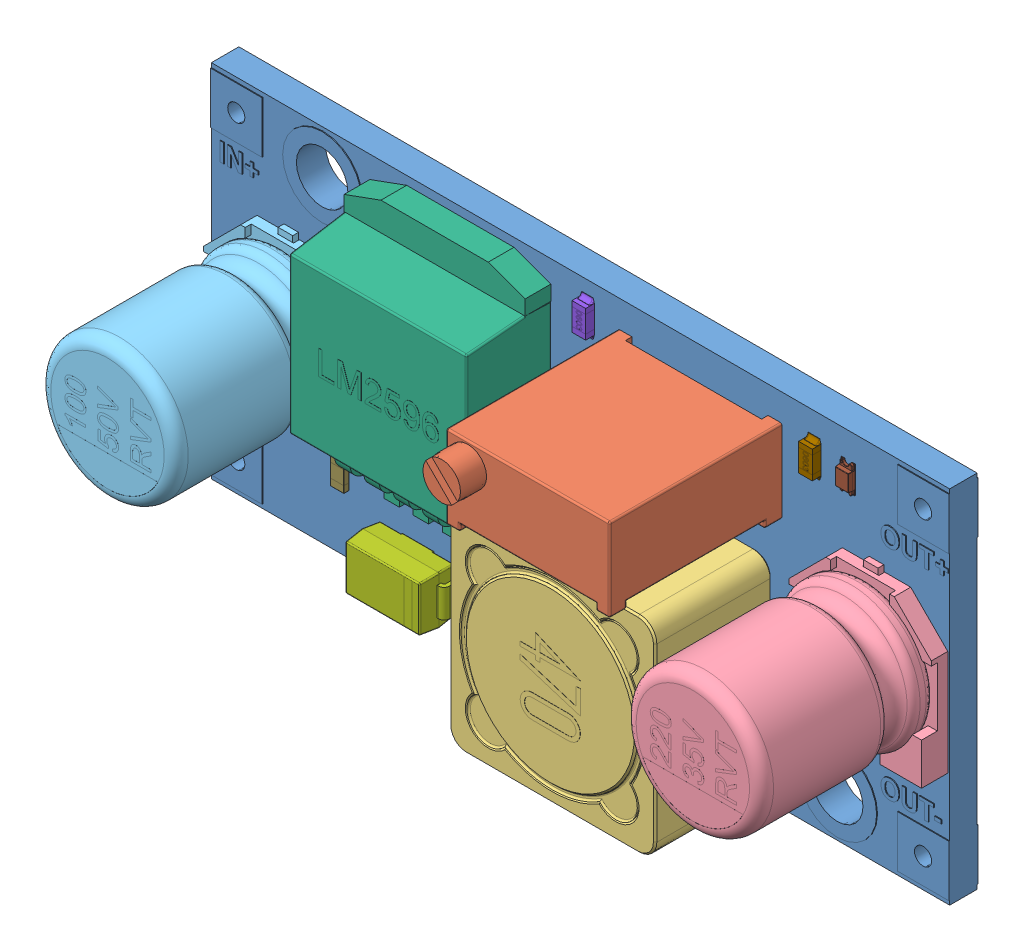
SolidWorks assembly LM2596 DC-DC StepDown Converter v1, configuration Default. Lengths in mm.
Overall size (43 21 14.15).
13 component instances, 12 part files, 0 mates.
Components (placement in the parent):
- LM2596 DC-DC StepDown Converter v1.step-1: LM2596 DC-DC StepDown Converter v1.step [Default] at origin size (43 21 14.15)
  - Board v5.step-1: Board v5.step [Default] at (0 -9.7327 -11.3327) x (1 0 0) z (0 -1 0) size (43 1.7 21)
  - Trimpot 3296W v1.step-1: Trimpot 3296W v1.step [Default] at (-14.54 7.2723 -9.7327) x (-1 0 0) z (0 0 1) size (9.56 4.83 14.15)
  - CDRH127_470M v1.step-1: CDRH127_470M v1.step [Default] at (-15.855 -2.8827 -9.7427) x (0 -1 0) z (0 0 1) size (12.76 12.29 7.41)
  - CAPSMD220-35 v1.step-1: CAPSMD220-35 v1.step [Default] at (-4.2601 1.0246 -9.7327) x (0 1 0) z (0 0 1) size (9 8.3 10.7)
  - CAPSMD100-50 v1.step-1: CAPSMD100-50 v1.step [Default] at (-38.35 0.7473 -9.7327) x (0 1 0) z (0 0 1) size (9 8.3 10.7)
  - TO-263BA v2.step-1: TO-263BA v2.step [Default] at (-31.9 -3.4327 -9.7327) size (10.64 15.85 4.81)
  - DO-214AC-DIOM5127X23N v1.step-1: DO-214AC-DIOM5127X23N v1.step [Default] at (-32.735 -7.9827 -9.7327) size (5.3 2.8 2.3)
  - Resistor 0603 v1.step-1: Resistor 0603 v1.step [Default] at (-19.95 10.2673 -9.7327) x (0 -1 0) z (-1 0 0) size (2.1 0.6 0.8)
  - Resistor 0603 v1 (1).step-1: Resistor 0603 v1 (1).step [Default] at (-6.75 9.7673 -9.7327) x (0 -1 0) z (-1 0 0) size (2.1 0.6 0.8)
  - CAP0603 v1.step-1: CAP0603 v1.step [Default] at (-21.085 5.9823 -9.7327) x (0 -1 0) z (0 0 1) size (1.61 0.81 0.31)
  - FCrth 150060BS55040 v1.step-1: FCrth 150060BS55040 v1.step [Default] at (-5.89 8.9773 -9.7327) x (0 -1 0) z (0 0 1) size (1.6 0.8 0.4)
  - CAP0603 v1 (1).step-1: CAP0603 v1 (1).step [Default] at (-35.385 -5.5177 -9.7327) x (0 -1 0) z (0 0 1) size (1.61 0.81 0.31)
